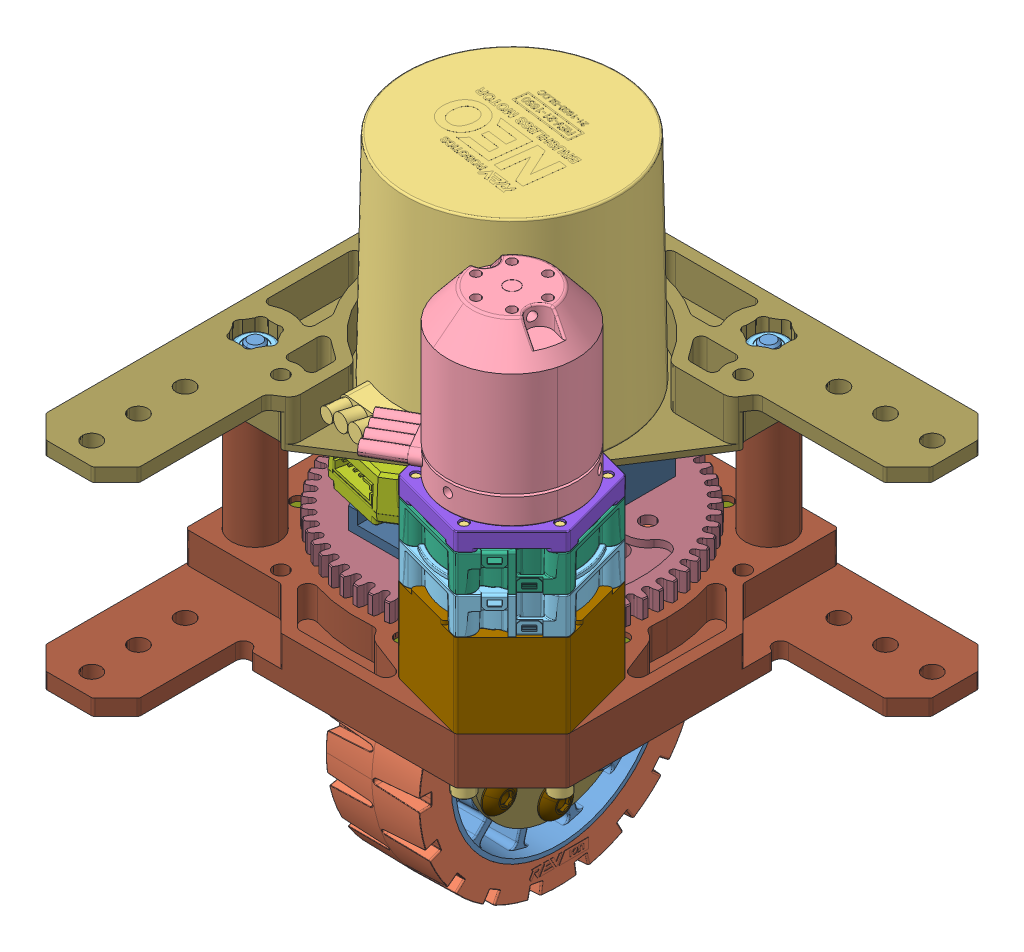
SolidWorks assembly REV-21-3005, configuration Default. Lengths in mm.
Overall size (142.9 171.46 142.9).
74 component instances, 41 part files, 0 mates.
Components (placement in the parent):
- REV-21-3005.STEP-1: REV-21-3005.STEP [Default] at origin size (142.9 171.46 142.9)
  - REV-21-3004.STEP-1: REV-21-3004.STEP [Default] x (0 0 -1) z (1 0 0) size (76.2 76.2 25.66)
    - REV-20-3003.STEP-1: REV-20-3003.STEP [Default] at origin size (67.63 67.63 25.4)
    - REV-21-3004-P01.STEP-1: REV-21-3004-P01.STEP [Default] x (0 0 -1) z (1 0 0) size (25.66 76.2 76.2)
  - REV-21-1650.STEP-1: REV-21-1650.STEP [Default] at (0 75.1 0) x (0.788011 0 -0.615661) z (0 -1 0) size (64.41 64.76 93.26)
  - REV-21-1651.STEP-1: REV-21-1651.STEP [Default] at (35.023 76.35 35.023) x (0 1 0) z (-0.258819 0 0.965926) size (56.01 42.91 43.01)
  - REV-41-1601.STEP-1: REV-41-1601.STEP [Default] at (35.023 67.85 35.023) x (-0.258819 0 -0.965926) z (0 1 0) size (43.57 38.28 17.88)
  - REV-41-1602.STEP-1: REV-41-1602.STEP [Default] at (35.023 77.85 35.023) x (-0.258819 0 -0.965926) z (0 1 0) size (43.57 38.28 17.88)
  - REV-41-1608.STEP-1: REV-41-1608.STEP [Default] at (35.023 80.35 35.023) x (0 0 1) z (0 -1 0) size (8.22 8.17 6)
  - REV-41-1607.STEP-1: REV-41-1607.STEP [Default] at (35.023 87.85 35.023) x (0.965926 0 0.258819) z (0.258819 0 -0.965926) size (43.67 5 38.01)
  - M3 BHCS SS_08mm Long.STEP-1: M3 BHCS SS_08mm Long.STEP [Default] at (22.9489 83.35 31.7878) x (-0.258819 0 0.965926) z (0 -1 0) size (5.7 5.7 9.66)
  - M3 BHCS SS_08mm Long.STEP-2: M3 BHCS SS_08mm Long.STEP [Default] at (47.0971 83.35 38.2582) x (0 0 1) z (0 -1 0) size (5.7 5.7 9.66)
  - 6812ZZ.STEP-1: 6812ZZ.STEP [Default] at (0 34.37 0) x (0.567918 0 0.823085) z (0 1 0) size (78 78 10)
  - REV-21-3005-P01.STEP-1: REV-21-3005-P01.STEP [Default] at (0 40.1638 0) x (1 0 0) z (0 1 0) size (133.1 133.1 12.7)
  - REV-21-3005-P02.STEP-1: REV-21-3005-P02.STEP [Default] at (0 73.5125 0) x (1 0 0) z (0 1 0) size (133.1 133.1 12.7)
  - REV-21-3005-P03.STEP-1: REV-21-3005-P03.STEP [Default] at (0 43.4975 0) x (1 0 0) z (0 -1 0) size (81.28 81.23 15.68)
  - REV-21-3005-P06.STEP-1: REV-21-3005-P06.STEP [Default] at (-22.86 28.125 0) x (-1 0 0) z (0 0 1) size (20.83 43.13 20.94)
  - REV-21-3005-P07.STEP-1: REV-21-3005-P07.STEP [Default] at (-13.485 0 0) x (0 1 0) z (0 0 1) size (56.88 16.86 56.92)
  - 6800ZZ.STEP-1: 6800ZZ.STEP [Default] at (-22.86 41.95 0) x (1 0 0) z (0 1 0) size (19 19 5)
  - MR106ZZ.STEP-1: MR106ZZ.STEP [Default] at (-22.86 14.55 0) x (1 0 0) z (0 1 0) size (10 10 3)
  - MR106ZZ.STEP-2: MR106ZZ.STEP [Default] at (-22.86 11.55 0) x (1 0 0) z (0 1 0) size (10 10 3)
  - REV-21-3005-P04.STEP-1: REV-21-3005-P04.STEP [Default] at (0 34.37 0) x (1 0 0) z (0 -1 0) size (16.68 50.74 40.72)
  - REV-21-3005-P05.STEP-1: REV-21-3005-P05.STEP [Default] at (0 34.37 0) x (1 0 0) z (0 -1 0) size (16.57 50.74 40.72)
  - REV-21-3005-P08.STEP-1: REV-21-3005-P08.STEP [Default] at (35.023 43.4975 35.023) x (1 0 0) z (0 1 0) size (22.81 22.24 25.89)
  - F688ZZ.STEP-1: F688ZZ.STEP [Default] at (0 42.6 0) x (1 0 0) z (0 -1 0) size (18 18 5)
  - REV-21-3005-P09.STEP-1: REV-21-3005-P09.STEP [Default] at (0 46.8312 0) x (-1 0 0) z (0 1 0) size (20.1 20.1 8.08)
  - REV-21-3005-P10.STEP-1: REV-21-3005-P10.STEP [Default] at (0 0 2.85) size (2 23.5 3)
  - REV-21-3005-P11.STEP-1: REV-21-3005-P11.STEP [Default] at (-22.86 50.0063 0) x (0 0 1) z (0 -1 0) size (30.48 30.33 8.74)
  - REV-11-1271.STEP-1: REV-11-1271.STEP [Default] at (0 71.5125 0) x (-0.224481 0 0.974478) z (0 -1 0) size (57.37 49.78 15.83)
  - 6701ZZ.STEP-1: 6701ZZ.STEP [Default] at (35.023 38.1638 35.023) x (1 0 0) z (0 -1 0) size (18 18 4)
  - 6701ZZ.STEP-2: 6701ZZ.STEP [Default] at (35.023 60.0563 35.023) x (1 0 0) z (0 -1 0) size (18 18 4)
  - REV-21-3005-P12.STEP-1: REV-21-3005-P12.STEP [Default] at (0 40.1638 0) x (1 0 0) z (0 1 0) size (42.15 42.15 23.69)
  - REV-21-3005-P13.STEP-1: REV-21-3005-P13.STEP [Default] at (0 46.0375 0) x (-1 0 0) z (0 1 0) size (31.75 57.15 29.98)
  - REV-21-3005-P14.STEP-1: REV-21-3005-P14.STEP [Default] at (-34.925 56.8381 34.925) x (1 0 0) z (0 -1 0) size (12.7 12.7 38.1)
  - REV-21-3005-P14.STEP-2: REV-21-3005-P14.STEP [Default] at (-34.925 56.8381 -34.925) x (0.982082 0 -0.188455) z (0 -1 0) size (12.7 12.7 38.1)
  - REV-21-3005-P14.STEP-3: REV-21-3005-P14.STEP [Default] at (34.925 56.8381 -34.925) x (0.918365 0 -0.395734) z (0 -1 0) size (12.7 12.7 38.1)
  - REV-21-3005-P15.STEP-1: REV-21-3005-P15.STEP [Default] at origin size (11.52 44.45 44.45)
  - F6900ZZ.STEP-1: F6900ZZ.STEP [Default] at (-11.2875 0 0) x (0 0 -1) z (1 0 0) size (25 25 6)
  - F6900ZZ.STEP-2: F6900ZZ.STEP [Default] at (10.0175 0 0) x (0 0 1) z (-1 0 0) size (25 25 6)
  - REV-21-3005-P18.STEP-1: REV-21-3005-P18.STEP [Default] x (0 0 -1) z (1 0 0) size (9.99 9.99 36.45)
  - REV-21-3005-P19.STEP-1: REV-21-3005-P19.STEP [Default] at (-17.272 34.37 0) x (0 1 0) z (1 0 0) size (15 15 2.98)
  - REV-21-3005-P19.STEP-2: REV-21-3005-P19.STEP [Default] at (13.0175 34.37 0) x (0 1 0) z (1 0 0) size (15 15 2.98)
  - #10 Button Head Cap Screws_0.375 Long.STEP-1: #10 Button Head Cap Screws_0.375 Long.STEP [Default] at (-36.5125 32.8498 -20.7566) x (0.837169 0 0.546944) z (0 -1 0) size (9.17 9.17 12.1)
  - #10 Button Head Cap Screws_0.375 Long.STEP-2: #10 Button Head Cap Screws_0.375 Long.STEP [Default] at (-22.86 49.7015 0) x (-1 0 0) z (0 1 0) size (9.17 9.17 12.1)
  - #10 Button Head Cap Screws_0.375 Long.STEP-3: #10 Button Head Cap Screws_0.375 Long.STEP [Default] at (-20.7566 32.8498 -36.5125) x (0.925243 0 0.379375) z (0 -1 0) size (9.17 9.17 12.1)
  - #10 Button Head Cap Screws_0.375 Long.STEP-4: #10 Button Head Cap Screws_0.375 Long.STEP [Default] at (22.6769 32.8498 -35.3519) x (0.985271 0 0.170998) z (0 -1 0) size (9.17 9.17 12.1)
  - #10 Button Head Cap Screws_0.375 Long.STEP-5: #10 Button Head Cap Screws_0.375 Long.STEP [Default] at (40.5689 32.9998 10.8704) x (0.997902 0 -0.064746) z (0 -1 0) size (9.17 9.17 12.1)
  - #10 Button Head Cap Screws_0.375 Long.STEP-6: #10 Button Head Cap Screws_0.375 Long.STEP [Default] at (10.8704 32.9998 40.5689) x (0.953572 0 -0.301166) z (0 -1 0) size (9.17 9.17 12.1)
  - #10 Button Head Cap Screws_0.375 Long.STEP-7: #10 Button Head Cap Screws_0.375 Long.STEP [Default] at (-35.3519 32.8498 22.6769) x (0.86157 0 -0.507639) z (0 -1 0) size (9.17 9.17 12.1)
  - #10 Button Head Cap Screws_0.500 Long.STEP-1: #10 Button Head Cap Screws_0.500 Long.STEP [Default] at (-15.6378 73.5798 -20.0155) x (0.775412 0 0.631456) z (0 -1 0) size (9.17 9.17 15.27)
  - #10 Button Head Cap Screws_0.500 Long.STEP-2: #10 Button Head Cap Screws_0.500 Long.STEP [Default] at (15.6378 73.5798 20.0155) x (0.880519 0 0.474011) z (0 -1 0) size (9.17 9.17 15.27)
  - #10 Button Head Cap Screws_1.000 Long.STEP-1: #10 Button Head Cap Screws_1.000 Long.STEP [Default] at (0.1002 -17.78 0) x (0 -0.825172 0.564882) z (1 0 0) size (9.17 9.17 27.97)
  - #10 Button Head Cap Screws_1.000 Long.STEP-2: #10 Button Head Cap Screws_1.000 Long.STEP [Default] at (0.1002 -8.89 15.3979) x (0 -0.904297 0.426903) z (1 0 0) size (9.17 9.17 27.97)
  - #10 Button Head Cap Screws_1.000 Long.STEP-3: #10 Button Head Cap Screws_1.000 Long.STEP [Default] at (0.1002 8.89 15.3979) x (0 -0.951295 0.308282) z (1 0 0) size (9.17 9.17 27.97)
  - #10 Button Head Cap Screws_1.000 Long.STEP-4: #10 Button Head Cap Screws_1.000 Long.STEP [Default] at (0.1002 17.78 0) x (0 -0.975889 0.218268) z (1 0 0) size (9.17 9.17 27.97)
  - #10 Button Head Cap Screws_1.000 Long.STEP-5: #10 Button Head Cap Screws_1.000 Long.STEP [Default] at (0.1002 8.89 -15.3979) x (0 -0.986324 0.164818) z (1 0 0) size (9.17 9.17 27.97)
  - #10 Button Head Cap Screws_1.000 Long.STEP-6: #10 Button Head Cap Screws_1.000 Long.STEP [Default] at (0.1002 -8.89 -15.3979) x (0 -0.987881 0.155215) z (1 0 0) size (9.17 9.17 27.97)
  - #10 Socket Head Cap Screws_2.000 Long.STEP-1: #10 Socket Head Cap Screws_2.000 Long.STEP [Default] at (-34.925 84.6137 34.925) x (0 0 -1) z (0 1 0) size (7.94 7.94 55.63)
  - #10 Socket Head Cap Screws_2.000 Long.STEP-2: #10 Socket Head Cap Screws_2.000 Long.STEP [Default] at (-34.925 84.6137 -34.925) x (-0.188455 0 -0.982082) z (0 1 0) size (7.94 7.94 55.63)
  - #10 Socket Head Cap Screws_2.000 Long.STEP-3: #10 Socket Head Cap Screws_2.000 Long.STEP [Default] at (34.925 84.6137 -34.925) x (-0.395734 0 -0.918365) z (0 1 0) size (7.94 7.94 55.63)
  - #10 Socket Head Cap Screws_1.000 Long.STEP-1: #10 Socket Head Cap Screws_1.000 Long.STEP [Default] at (-22.606 43.895 14.351) x (-0.561714 0 -0.827332) z (0 1 0) size (7.94 7.94 30.23)
  - #10 Socket Head Cap Screws_1.000 Long.STEP-2: #10 Socket Head Cap Screws_1.000 Long.STEP [Default] at (-22.606 43.895 -14.351) x (-0.707564 0 -0.70665) z (0 1 0) size (7.94 7.94 30.23)
  - #10 Socket Head Cap Screws_1.000 Long.STEP-3: #10 Socket Head Cap Screws_1.000 Long.STEP [Default] at (22.606 43.895 14.351) x (-0.843262 0 -0.537503) z (0 1 0) size (7.94 7.94 30.23)
  - #10 Socket Head Cap Screws_1.000 Long.STEP-4: #10 Socket Head Cap Screws_1.000 Long.STEP [Default] at (22.606 43.895 -14.351) x (-0.94577 0 -0.324837) z (0 1 0) size (7.94 7.94 30.23)
  - #10 Socket Head Cap Screws_2.000 Long.STEP-4: #10 Socket Head Cap Screws_2.000 Long.STEP [Default] at (-30.0355 0 0) x (0 0.886241 -0.463225) z (-1 0 0) size (7.94 7.94 55.63)
  - M3 SHCS SS_60mm Long.STEP-1: M3 SHCS SS_60mm Long.STEP [Default] at (21.9591 55.9637 48.0869) x (1 0 0) z (0 -1 0) size (5.5 5.5 63.01)
  - M3 SHCS SS_60mm Long.STEP-2: M3 SHCS SS_60mm Long.STEP [Default] at (39.8047 55.9637 52.8687) x (0.982082 0 -0.188455) z (0 -1 0) size (5.5 5.5 63.01)
  - M3 SHCS SS_60mm Long.STEP-3: M3 SHCS SS_60mm Long.STEP [Default] at (52.8687 55.9637 39.8047) x (0.918365 0 -0.395734) z (0 -1 0) size (5.5 5.5 63.01)
  - M3 SHCS SS_60mm Long.STEP-4: M3 SHCS SS_60mm Long.STEP [Default] at (48.0869 55.9637 21.9591) x (0.8 0 -0.6) z (0 -1 0) size (5.5 5.5 63.01)
  - M3 SHCS SS_25mm Long.STEP-1: M3 SHCS SS_25mm Long.STEP [Default] at (17.1773 71.5563 30.2413) x (1 0 0) z (0 -1 0) size (5.5 5.5 28.01)
  - M3 SHCS SS_25mm Long.STEP-2: M3 SHCS SS_25mm Long.STEP [Default] at (30.2413 71.5563 17.1773) x (0.982082 0 -0.188455) z (0 -1 0) size (5.5 5.5 28.01)
  - REV-29-1016.STEP-1: REV-29-1016.STEP [Default] at (-34.925 79.0631 34.925) size (11.04 4.39 9.57)
  - REV-29-1016.STEP-2: REV-29-1016.STEP [Default] at (-34.925 79.0631 -34.925) x (0.965926 0 -0.258819) z (0.258819 0 0.965926) size (11.04 4.39 9.57)
  - REV-29-1016.STEP-3: REV-29-1016.STEP [Default] at (34.925 79.0631 -34.925) x (0.866025 0 -0.5) z (0.5 0 0.866025) size (11.04 4.39 9.57)
